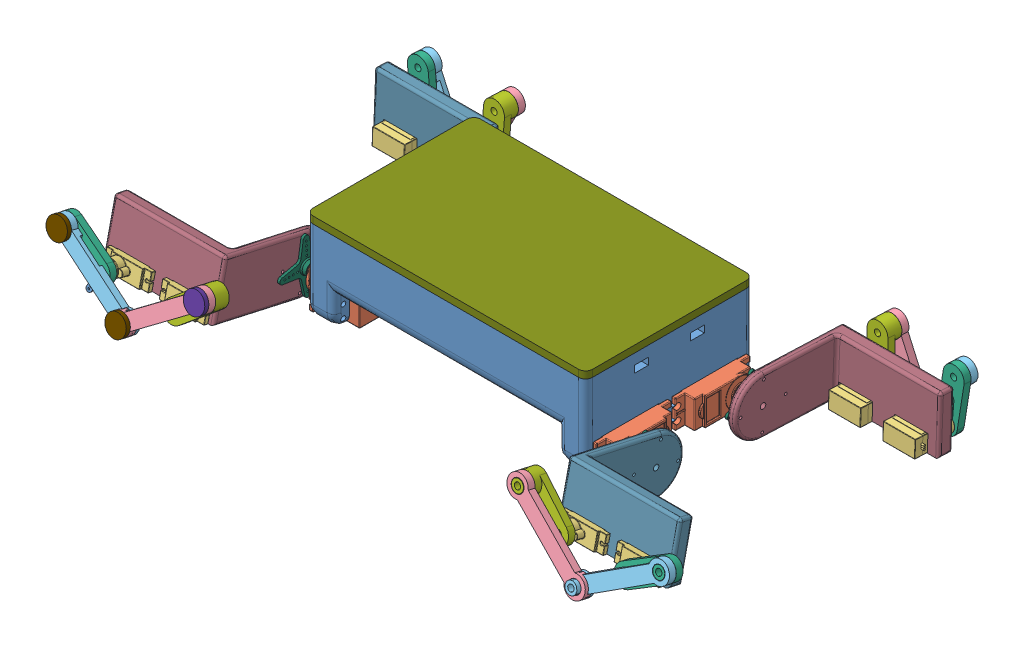
SolidWorks assembly ASSY2, configuration Default. Lengths in mm.
Overall size (448.61 106.34 262.67).
50 component instances, 19 part files, 76 mates.
Components (placement in the parent):
- part1-1: part1 [Default] at (0 487.6228 0) size (200.21 60 120)
- Servo MG996R-2: Servo MG996R [Predeterminado] at (-73.4 487.6228 48.3) x (0 0 -1) z (0 1 0) size (53.6 47.6 20)
- Servo-MG90S-1: Servo-MG90S [Default] at (-142.75 473.3283 84.1782) x (1 0 0) z (0 -0.975912 0.218163) size (32.2 32.5 12.4)
- Servo-MG90S-2: Servo-MG90S [Default] at (-182.75 473.3283 84.1782) x (-1 0 0) z (0 0.975912 -0.218163) size (32.2 32.5 12.4)
- legpart1-1: legpart1 [Default] at (-114.3085 500.4086 118.087) x (-0.808135 -0.574809 0.128497) z (0 0.218163 0.975912) size (75 15 5)
- legpart2-1: legpart2 [Default] at (-213.9956 495.9485 116.7273) x (0.853315 -0.508837 0.113749) z (0 0.218163 0.975912) size (75 15 10)
- legpart3-1: legpart3 [Default] at (-188 480.244 115.1146) x (-0.866519 0.487122 -0.108895) z (0 0.218163 0.975912) size (45 15 10)
- legpart4-1: legpart4 [Default] at (-137.5 479.655 112.4796) x (0.773049 0.619067 -0.138391) z (0 0.218163 0.975912) size (45 15 15.1)
- Arduino Mega.step-1: Arduino Mega.step [Default] at (-11.5076 498.6228 34.714) x (0.34202 0 -0.939693) z (0.939693 0 0.34202) size (114.59 14.37 81.93)
  - ARDUINO MEGA_1.step-1: ARDUINO MEGA_1.step [Default] at origin size (114.59 14.37 81.93)
- 18650BatteryCase v6.step-1: 18650BatteryCase v6.step [Default] at (14.4936 492.6228 -12.397) x (1 0 0) z (0 1 0) size (76.1 23.18 18.4)
- 18650 battery-1: 18650 battery [Default] at (84.4936 502.6228 -24.397) x (0 0 1) z (0 -1 0) size (18.4 65 18.4)
- 18650 battery-3: 18650 battery [Default] at (84.4936 502.6228 -0.397) x (0 0 -1) z (0 1 0) size (18.4 65 18.4)
- 18650BatteryCase v6.step-3: 18650BatteryCase v6.step [Default] at (14.4936 492.6228 9.103) x (1 0 0) z (0 1 0) size (76.1 23.18 18.4)
- HC-05-1: HC-05 [Default] at (-0.9997 492.6228 -7.5776) x (-0.021576 0 -0.999767) z (0.999767 0 -0.021576) size (42.58 6.55 16)
- matrix-1: matrix [Default] at (54 492.6228 28.5) size (82 14.01 53)
- part2L-7: part2L [Default] at (-125.75 477.6228 38.3) x (0 0.218163 0.975912) z (-1 0 0) size (82.34 40 80)
- part2R-7: part2R [Default] at (-125.75 477.6228 -38.3) x (0 -0.039775 -0.999209) z (-1 0 0) size (82.34 40 80)
- Servo MG996R-8: Servo MG996R [Predeterminado] at (-73.4 467.6228 -48.3) x (0 0 1) z (0 -1 0) size (53.6 47.6 20)
- Servo MG996R-9: Servo MG996R [Predeterminado] at (73.4 487.6228 -48.3) x (0 0 1) z (0 1 0) size (53.6 47.6 20)
- Servo MG996R-10: Servo MG996R [Predeterminado] at (73.4 467.6228 48.3) x (0 0 -1) z (0 -1 0) size (53.6 47.6 20)
- Servo Control Horns-1: Servo Control Horns [4 Arm] at (-121 467.3785 37.9577) x (0 -0.999442 -0.033391) z (-1 0 0) size (39 39 5.5)
- Servo Control Horns-2: Servo Control Horns [4 Arm] at (-121 477.2455 -28.057) x (0 -0.036806 0.999322) z (-1 0 0) size (39 39 5.5)
- Servo-MG90S-13: Servo-MG90S [Default] at (-182.75 461.6904 -81.5367) x (-1 0 0) z (0 -0.999209 0.039775) size (32.2 32.5 12.4)
- Servo-MG90S-14: Servo-MG90S [Default] at (-143.75 461.6904 -81.5367) x (1 0 0) z (0 0.999209 -0.039775) size (32.2 32.5 12.4)
- legpart4-8: legpart4 [Default] at (-138.5 460.5369 -110.5137) x (0.042245 0.998317 -0.03974) z (0 -0.039775 -0.999209) size (45 15 15.1)
- legpart1-8: legpart1 [Default] at (-137.2327 489.8898 -126.6941) x (-0.450757 -0.89194 0.035505) z (0 0.039775 0.999209) size (75 15 5)
- legpart2-8: legpart2 [Default] at (-191.7269 490.0821 -116.6938) x (0.457481 -0.888516 0.035369) z (0 -0.039775 -0.999209) size (75 15 10)
- legpart3-8: legpart3 [Default] at (-188 460.5369 -110.5137) x (-0.124231 0.991468 -0.039467) z (0 -0.039775 -0.999209) size (45 15 10)
- Servo Control Horns-3: Servo Control Horns [4 Arm] at (121 487.8563 -37.7196) x (0 0.998396 0.056621) z (1 0 0) size (39 39 5.5)
- Servo Control Horns-5: Servo Control Horns [4 Arm] at (121 478 28.057) x (0 0.036806 -0.999322) z (1 0 0) size (39 39 5.5)
- part2R-12: part2R [Default] at (125.75 477.6228 38.3) x (0 0.218163 0.975912) z (1 0 0) size (82.34 40 80)
- part2L-13: part2L [Default] at (125.75 477.6228 -38.3) x (0 -0.039775 -0.999209) z (1 0 0) size (82.34 40 80)
- legpart4-14: legpart4 [Default] at (138.5 460.5369 -110.5137) x (-0.042245 0.998317 -0.03974) z (0 -0.039775 -0.999209) size (45 15 15.1)
- legpart3-14: legpart3 [Default] at (188 460.5369 -110.5137) x (0.124231 0.991468 -0.039467) z (0 -0.039775 -0.999209) size (45 15 10)
- Servo-MG90S-25: Servo-MG90S [Default] at (182.75 461.6904 -81.5367) x (1 0 0) z (0 0.999209 -0.039775) size (32.2 32.5 12.4)
- Servo-MG90S-26: Servo-MG90S [Default] at (143.75 461.6904 -81.5367) x (-1 0 0) z (0 -0.999209 0.039775) size (32.2 32.5 12.4)
- legpart1-14: legpart1 [Default] at (137.2327 490.0887 -121.698) x (0.450757 -0.89194 0.035505) z (0 -0.039775 -0.999209) size (75 15 5)
- legpart2-14: legpart2 [Default] at (191.7269 490.0821 -116.6938) x (-0.457481 -0.888516 0.035369) z (0 -0.039775 -0.999209) size (75 15 10)
- Servo-MG90S-27: Servo-MG90S [Default] at (142.75 473.3283 84.1782) x (-1 0 0) z (0 0.975912 -0.218163) size (32.2 32.5 12.4)
- Servo-MG90S-28: Servo-MG90S [Default] at (182.75 473.3283 84.1782) x (1 0 0) z (0 -0.975912 0.218163) size (32.2 32.5 12.4)
- legpart3-15: legpart3 [Default] at (188 480.244 115.1146) x (0.866519 0.487122 -0.108895) z (0 0.218163 0.975912) size (45 15 10)
- legpart2-15: legpart2 [Default] at (213.9956 495.9485 116.7273) x (-0.853315 -0.508837 0.113749) z (0 0.218163 0.975912) size (75 15 10)
- legpart1-15: legpart1 [Default] at (114.3085 501.4994 122.9666) x (0.808135 -0.574809 0.128497) z (0 -0.218163 -0.975912) size (75 15 5)
- legpart4-15: legpart4 [Default] at (137.5 479.655 112.4796) x (-0.773049 0.619067 -0.138391) z (0 0.218163 0.975912) size (45 15 15.1)
- 사본 파트1^ASSY2-1: 사본 파트1^ASSY2 [Default] at (0 814.6335 0) x (1 0 0) z (0 1 0) size (200 120 10) (virtual)
- legpart5-1: legpart5 [Default] at (-114.3085 502.1539 125.8943) x (-0.886163 0.452213 -0.101091) z (-0.463375 -0.864817 0.193328) size (15 18 15)
- legpart6-1: legpart6 [Default] at (-162.7967 467.6654 133.6042) x (0.999961 0.008577 -0.001917) z (-0.008789 0.975875 -0.218154) size (15 13 15)
- legpart6-2: legpart6 [Default] at (-213.9956 497.6938 124.5346) x (0.324849 0.922985 -0.206331) z (-0.945766 0.317024 -0.07087) size (15 13 15)
- servo horn 1 v2.step-1: servo horn 1 v2.step [Default] at (-188 480.4185 115.8953) x (0.877073 -0.468786 0.104796) z (-0.480356 -0.855947 0.191345) size (7.2 3.7 21.2)
Mates (geometry in assembly coordinates):
- 일치5: coincident: plane of part1-1 through (0 487.6228 0) normal (0 -1 0); plane of Servo MG996R-2 through (-110 487.6228 48.3) normal (0 1 0)
- 일치22: coincident: plane of Servo-MG90S-1 through (-137.5 479.655 112.4796) normal (0 0.218163 0.975912); plane of legpart4-1 through (-137.5 479.655 112.4796) normal (0 -0.218163 -0.975912)
- 동심5: concentric: cylinder of Servo-MG90S-1 through (-137.5 479.8731 113.4556) axis (0 0.218163 0.975912) radius 1.25; cylinder of legpart4-1 through (-137.5 480.7458 117.3592) axis (0 -0.218163 -0.975912) radius 2.5
- 동심6: concentric: cylinder of legpart1-1 through (-114.3085 501.4994 122.9666) axis (0 -0.218163 -0.975912) radius 4.5; cylinder of legpart4-1 through (-114.3085 501.5212 123.0642) axis (0 -0.218163 -0.975912) radius 4.25
- 일치23: coincident: plane of legpart1-1 through (-114.3085 500.4086 118.087) normal (0 -0.218163 -0.975912); plane of legpart4-1 through (-114.3085 500.4086 118.087) normal (0 0.218163 0.975912)
- 동심7: concentric: cylinder of Servo-MG90S-2 through (-188 479.8731 113.4556) axis (0 0.218163 0.975912) radius 1.25; cylinder of legpart3-1 through (-188 481.3348 119.9942) axis (0 -0.218163 -0.975912) radius 2.5
- 동심8: concentric: cylinder of legpart2-1 through (-213.9956 497.0393 121.6069) axis (0 -0.218163 -0.975912) radius 4.5; cylinder of legpart3-1 through (-213.9956 497.0393 121.6069) axis (0 -0.218163 -0.975912) radius 4.25
- 일치25: coincident: plane of legpart2-1 through (-213.9956 495.9485 116.7273) normal (0 -0.218163 -0.975912); plane of legpart3-1 through (-188 481.3348 119.9942) normal (0 0.218163 0.975912)
- 동심9: concentric: cylinder of legpart1-1 through (-162.7967 467.0109 130.6764) axis (0 -0.218163 -0.975912) radius 4.5; cylinder of legpart2-1 through (-162.7967 467.5999 133.3114) axis (0 -0.218163 -0.975912) radius 4.25
- 거리7: distance = 20 mm: plane of Arduino Mega.step-1/ARDUINO MEGA_1.step-1 through (-40 500.4228 -52) normal (-1 0 0); plane of part1-1 through (-20 512.6228 -45) normal (-1 0 0)
- 일치31: coincident: plane of part1-1 through (0 492.6228 0) normal (0 1 0); plane of 18650BatteryCase v6.step-1 through (52.4936 492.6228 -23.147) normal (0 -1 0)
- 거리8: distance = 10 mm: plane of 18650BatteryCase v6.step-1 through (14.4936 492.6228 -12.397) normal (0 1 0); plane of 18650 battery-1 through (84.4936 502.6228 -24.397) normal (0 -1 0)
- 거리9: distance = 12 mm: plane of 18650 battery-1 through (84.4936 502.6228 -24.397) normal (0 0 1); plane of 18650BatteryCase v6.step-1 through (14.4936 492.6228 -12.397) normal (0 0 -1)
- 거리10: distance = 70 mm: plane of 18650 battery-1 through (84.4936 502.6228 -24.397) normal (-1 0 0); plane of 18650BatteryCase v6.step-1 through (14.4936 492.6228 -12.397) normal (1 0 0)
- 일치33: coincident: plane of part1-1 through (0 492.6228 0) normal (0 1 0); plane of matrix-1 through (54 492.6228 28.5) normal (0 -1 0)
- 일치34: coincident: plane of part1-1 through (95 527.6228 -55) normal (-1 0 0); plane of matrix-1 through (95 506.6269 2) normal (1 0 0)
- 일치35: coincident: plane of part1-1 through (-95 527.6228 55) normal (0 0 -1); plane of matrix-1 through (95 506.6269 55) normal (0 0 1)
- 일치36: coincident: plane of part1-1 through (0 492.6228 0) normal (0 1 0); plane of HC-05-1 through (-0.9997 492.6228 -7.5776) normal (0 -1 0)
- 일치38: coincident: plane of part1-1 through (0 487.6228 0) normal (1 0 0); plane of assembly through (0 0 0) normal (1 0 0)
- 일치39: coincident: plane of part1-1 through (-100 492.6228 -60) normal (0 0 -1); plane of Arduino Mega.step-1/ARDUINO MEGA_1.step-1 through (-34 500.9228 -60) normal (0 0 -1)
- 일치40: coincident: plane of part1-1 through (-62.5 498.6228 12.1502) normal (0 1 0); plane of Arduino Mega.step-1/ARDUINO MEGA_1.step-1 through (-44 498.6228 -52) normal (0 -1 0)
- 일치42: coincident: plane of Servo-MG90S-2 through (-182.75 477.3643 102.2326) normal (0 -0.218163 -0.975912); plane of part2L-7 through (-125.75 491.2222 99.1347) normal (0 0.218163 0.975912)
- 일치44: coincident: plane of Servo-MG90S-2 through (-182.75 479.3789 82.8256) normal (0 0.975912 -0.218163); plane of part2L-7 through (-194.75 481.2333 91.1208) normal (0 -0.975912 0.218163)
- 일치45: coincident: plane of Servo-MG90S-1 through (-142.75 479.3789 82.8256) normal (0 0.975912 -0.218163); plane of part2L-7 through (-130.75 481.2333 91.1208) normal (0 -0.975912 0.218163)
- 일치46: coincident: plane of Servo-MG90S-1 through (-142.75 477.3643 102.2326) normal (0 -0.218163 -0.975912); plane of part2L-7 through (-125.75 491.2222 99.1347) normal (0 0.218163 0.975912)
- 거리11: distance = 0.5 mm: plane of Servo-MG90S-1 through (-154.25 471.5088 103.5415) normal (-1 0 0); plane of part2L-7 through (-154.75 469.5223 93.7388) normal (1 0 0)
- 거리12: distance = 0.5 mm: plane of part2L-7 through (-194.75 469.5223 93.7388) normal (1 0 0); plane of Servo-MG90S-2 through (-194.25 483.2197 100.9236) normal (-1 0 0)
- 동심14: concentric: cylinder of Servo MG996R-2 through (-114.1 477.6228 38.3) axis (-1 0 0) radius 1.3; cylinder of Servo Control Horns-1 through (-122.75 477.6228 38.3) axis (1 0 0) radius 1.25
- 일치47: coincident: plane of Servo MG996R-2 through (-121 477.6228 38.3) normal (-1 0 0); plane of Servo Control Horns-1 through (-121 467.3785 37.9577) normal (1 0 0)
- 일치48: coincident: plane of part2L-7 through (-122.75 477.6228 38.3) normal (1 0 0); plane of Servo Control Horns-1 through (-122.75 467.3785 37.9577) normal (-1 0 0)
- 동심16: concentric: cylinder of part2L-7 through (-122.75 477.6228 38.3) axis (-1 0 0) radius 2; cylinder of Servo Control Horns-1 through (-122.75 477.6228 38.3) axis (1 0 0) radius 1.25
- 동심17: concentric: cylinder of Servo MG996R-8 through (-114.1 477.6228 -38.3) axis (-1 0 0) radius 1.3; cylinder of Servo Control Horns-2 through (-122.75 477.6228 -38.3) axis (1 0 0) radius 1.25
- 일치49: coincident: plane of Servo MG996R-8 through (-121 477.6228 -38.3) normal (-1 0 0); plane of Servo Control Horns-2 through (-121 477.2455 -28.057) normal (1 0 0)
- 동심18: concentric: cylinder of part2R-7 through (-122.75 477.6228 -38.3) axis (-1 0 0) radius 2; cylinder of Servo Control Horns-2 through (-122.75 477.6228 -38.3) axis (1 0 0) radius 1.25
- 일치50: coincident: plane of part2R-7 through (-122.75 477.6228 -38.3) normal (1 0 0); plane of Servo Control Horns-2 through (-122.75 477.2455 -28.057) normal (-1 0 0)
- 일치51: coincident: plane of Servo-MG90S-14 through (-138.5 460.5369 -110.5137) normal (0 -0.039775 -0.999209); plane of legpart4-8 through (-138.5 460.5369 -110.5137) normal (0 0.039775 0.999209)
- 동심19: concentric: cylinder of Servo-MG90S-14 through (-138.5 460.4972 -111.5129) axis (0 -0.039775 -0.999209) radius 1.25; cylinder of legpart4-8 through (-138.5 460.3381 -115.5098) axis (0 0.039775 0.999209) radius 2.5
- 동심20: concentric: cylinder of legpart4-8 through (-137.2327 489.8858 -126.794) axis (0 0.039775 0.999209) radius 4.25; cylinder of legpart1-8 through (-137.2327 490.0887 -121.698) axis (0 -0.039775 -0.999209) radius 4.5
- 일치52: coincident: plane of legpart4-8 through (-137.2327 490.0887 -121.698) normal (0 -0.039775 -0.999209); plane of legpart1-8 through (-137.2327 490.0887 -121.698) normal (0 0.039775 0.999209)
- 일치53: coincident: plane of Servo-MG90S-13 through (-188 460.5369 -110.5137) normal (0 -0.039775 -0.999209); plane of legpart3-8 through (-188 460.5369 -110.5137) normal (0 0.039775 0.999209)
- 동심21: concentric: cylinder of Servo-MG90S-13 through (-188 460.4972 -111.5129) axis (0 -0.039775 -0.999209) radius 1.25; cylinder of legpart3-8 through (-188 460.3381 -115.5098) axis (0 0.039775 0.999209) radius 2.5
- 동심22: concentric: cylinder of legpart2-8 through (-191.7269 489.8832 -121.6898) axis (0 0.039775 0.999209) radius 4.5; cylinder of legpart3-8 through (-191.7269 489.8832 -121.6898) axis (0 0.039775 0.999209) radius 4.25
- 일치54: coincident: plane of legpart2-8 through (-191.7269 490.0821 -116.6938) normal (0 0.039775 0.999209); plane of legpart3-8 through (-188 460.3381 -115.5098) normal (0 -0.039775 -0.999209)
- 동심23: concentric: cylinder of legpart1-8 through (-164.2781 436.5723 -119.5677) axis (0 -0.039775 -0.999209) radius 4.5; cylinder of legpart2-8 through (-164.2781 436.3734 -124.5637) axis (0 0.039775 0.999209) radius 4.25
- 일치55: coincident: plane of part2R-7 through (-130.75 467.5474 -90.2766) normal (0 -0.999209 0.039775); plane of Servo-MG90S-14 through (-143.75 467.8855 -81.7833) normal (0 0.999209 -0.039775)
- 거리13: distance = 0.5 mm: plane of Servo-MG90S-14 through (-155.25 466.9498 -100.2607) normal (-1 0 0); plane of part2R-7 through (-154.75 467.5474 -90.2766) normal (1 0 0)
- 일치56: coincident: plane of part2R-7 through (-130.75 467.5474 -90.2766) normal (0 -0.999209 0.039775); plane of Servo-MG90S-14 through (-143.75 467.8855 -81.7833) normal (0 0.999209 -0.039775)
- 일치57: coincident: plane of part2R-7 through (-125.75 475.1433 -100.5869) normal (0 -0.039775 -0.999209); plane of Servo-MG90S-14 through (-143.75 460.9546 -100.022) normal (0 0.039775 0.999209)
- 거리14: distance = 0.5 mm: plane of Servo-MG90S-13 through (-194.25 454.9593 -99.7834) normal (-1 0 0); plane of part2R-7 through (-194.75 467.5474 -90.2766) normal (1 0 0)
- 일치58: coincident: plane of part2R-7 through (-194.75 467.5474 -90.2766) normal (0 -0.999209 0.039775); plane of Servo-MG90S-13 through (-182.75 467.8855 -81.7833) normal (0 0.999209 -0.039775)
- 일치59: coincident: plane of part2R-7 through (-125.75 475.1433 -100.5869) normal (0 -0.039775 -0.999209); plane of Servo-MG90S-13 through (-182.75 460.9546 -100.022) normal (0 0.039775 0.999209)
- 동심33: concentric: cylinder of Servo Control Horns-3 through (122.75 477.6228 -38.3) axis (-1 0 0) radius 1.25; cylinder of part2L-13 through (122.75 477.6228 -38.3) axis (1 0 0) radius 2
- 동심35: concentric: cylinder of Servo Control Horns-5 through (122.75 477.6228 38.3) axis (-1 0 0) radius 1.25; cylinder of part2R-12 through (122.75 477.6228 38.3) axis (1 0 0) radius 2
- 동심37: concentric: cylinder of Servo MG996R-10 through (114.1 477.6228 38.3) axis (1 0 0) radius 1.3; cylinder of Servo Control Horns-5 through (122.75 477.6228 38.3) axis (-1 0 0) radius 1.25
- 일치71: coincident: plane of Servo MG996R-10 through (121 477.6228 38.3) normal (1 0 0); plane of Servo Control Horns-5 through (121 478 28.057) normal (-1 0 0)
- 동심38: concentric: cylinder of Servo MG996R-9 through (114.1 477.6228 -38.3) axis (1 0 0) radius 1.3; cylinder of Servo Control Horns-3 through (122.75 477.6228 -38.3) axis (-1 0 0) radius 1.25
- 일치72: coincident: plane of Servo MG996R-9 through (121 477.6228 -38.3) normal (1 0 0); plane of Servo Control Horns-3 through (121 487.8563 -37.7196) normal (-1 0 0)
- 일치73: coincident: plane of Servo Control Horns-3 through (122.75 487.8563 -37.7196) normal (1 0 0); plane of part2L-13 through (122.75 477.6228 -38.3) normal (-1 0 0)
- 일치74: coincident: plane of part2L-13 through (130.75 467.5474 -90.2766) normal (0 -0.999209 0.039775); plane of Servo-MG90S-26 through (143.75 467.8855 -81.7833) normal (0 0.999209 -0.039775)
- 일치75: coincident: plane of part2R-12 through (130.75 481.2333 91.1208) normal (0 -0.975912 0.218163); plane of Servo-MG90S-27 through (142.75 479.3789 82.8256) normal (0 0.975912 -0.218163)
- 일치76: coincident: plane of Servo Control Horns-5 through (122.75 478 28.057) normal (1 0 0); plane of part2R-12 through (122.75 477.6228 38.3) normal (-1 0 0)
- 일치77: coincident: plane of part1-1 through (0 487.6228 0) normal (0 -1 0); plane of Servo MG996R-8 through (-110 487.6228 -48.3) normal (0 1 0)
- 일치81: coincident: plane of part1-1 through (100 492.6228 -60) normal (1 0 0); plane of 사본 파트1^ASSY2-1 through (100 532.6228 -55) normal (1 0 0)
- 일치82: coincident: plane of part1-1 through (-100 492.6228 60) normal (0 0 1); plane of 사본 파트1^ASSY2-1 through (-95 532.6228 60) normal (0 0 1)
- 거리16: distance = 0.5 mm: plane of Servo MG996R-2 through (-110 487.6228 8) normal (0 0 -1); plane of part1-1 through (0 467.6228 7.5) normal (0 0 1)
- 거리17: distance = 0.5 mm: plane of Servo MG996R-8 through (-110 467.6228 -8) normal (0 0 1); plane of part1-1 through (0 467.6228 -7.5) normal (0 0 -1)
- 동심40: concentric: cylinder of legpart4-1 through (-114.3085 493.6456 87.8338) axis (0 0.218163 0.975912) radius 2.25; cylinder of legpart5-1 through (-114.3085 498.227 108.3279) axis (0 0.218163 0.975912) radius 2
- 일치84: coincident: plane of legpart1-1 through (-114.3085 501.4994 122.9666) normal (0 0.218163 0.975912); plane of legpart5-1 through (-114.3085 501.4994 122.9666) normal (0 -0.218163 -0.975912)
- 동심42: concentric: cylinder of legpart2-1 through (-162.7967 463.673 115.745) axis (0 0.218163 0.975912) radius 2.25; cylinder of legpart6-1 through (-162.7967 464.8292 120.9173) axis (0 0.218163 0.975912) radius 2
- 일치86: coincident: plane of legpart1-1 through (-114.3085 501.4994 122.9666) normal (0 0.218163 0.975912); plane of legpart6-1 through (-162.7967 467.0109 130.6764) normal (0 -0.218163 -0.975912)
- 동심43: concentric: cylinder of legpart3-1 through (-213.9956 488.3128 82.5704) axis (0 0.218163 0.975912) radius 2.25; cylinder of legpart6-2 through (-213.9956 494.8577 111.8478) axis (0 0.218163 0.975912) radius 2
- 일치87: coincident: plane of legpart2-1 through (-213.9956 497.0393 121.6069) normal (0 0.218163 0.975912); plane of legpart6-2 through (-213.9956 497.0393 121.6069) normal (0 -0.218163 -0.975912)
- 일치88: coincident: plane of part1-1 through (-100 492.6228 -60) normal (-1 0 0); plane of Servo MG996R-2 through (-100 487.6228 54.95) normal (1 0 0)
- 일치90: coincident: plane of Servo-MG90S-2 through (-188 480.4185 115.8953) normal (0 0.218163 0.975912); plane of servo horn 1 v2.step-1 through (-188 480.4185 115.8953) normal (0 -0.218163 -0.975912)
- 동심44: concentric: cylinder of Servo-MG90S-2 through (-188 479.8731 113.4556) axis (0 0.218163 0.975912) radius 1.25; cylinder of servo horn 1 v2.step-1 through (-188 480.4185 115.8953) axis (0 0.218163 0.975912) radius 1.1
- 일치91: coincident: plane of legpart3-1 through (-201.8643 488.4743 115.3241) normal (0 -0.218163 -0.975912); plane of servo horn 1 v2.step-1 through (-191.3625 474.6887 118.4058) normal (0 0.218163 0.975912)
